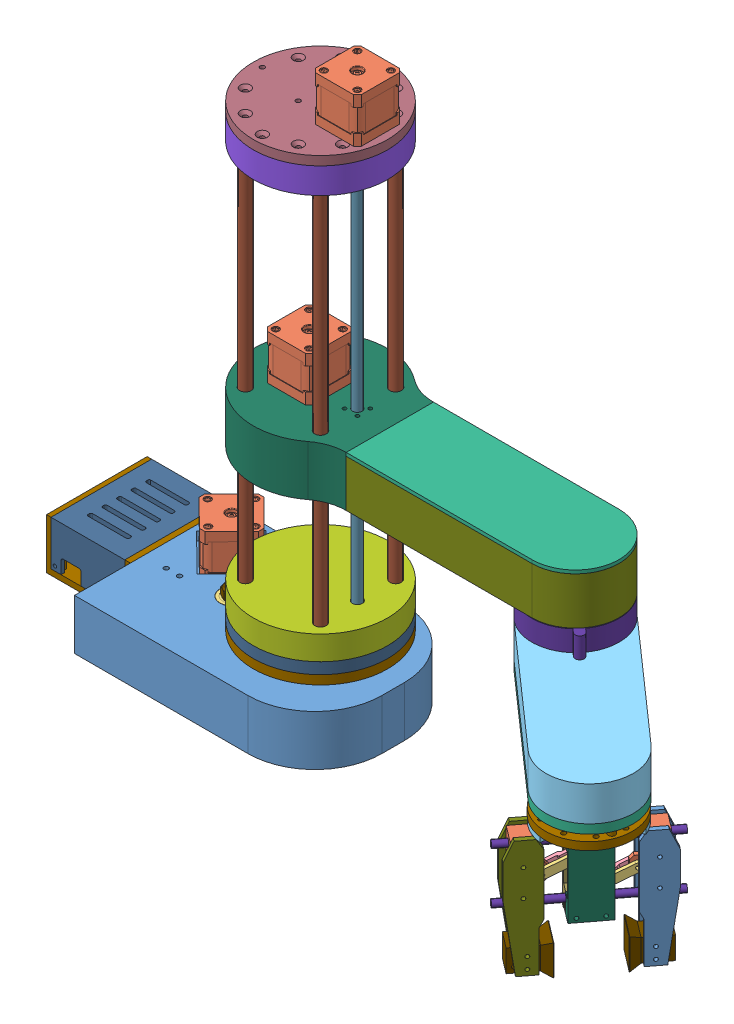
SolidWorks assembly SCARA Robot, configuration SCARA Robot. Lengths in mm.
Overall size (616.01 508 221.86).
112 component instances, 59 part files, 217 mates.
Components (placement in the parent):
- Base-1: Base [Base] at origin size (215 45 140)
- Stepper NEMA 17 -  20mm shaft-1: Stepper NEMA 17 -  20mm shaft [Stepper NEMA 17 -  20mm shaft] at (-89.369 63.0261 0.1561) x (-0.712104 0 -0.702074) z (0 -1 0) size (41 41 60)
- Ball Bearing 608 - 8x22x7mm-2: Ball Bearing 608 - 8x22x7mm [Ball Bearing 608 - 8x22x7mm] at (-36.5 3 0) x (0.982643 0 -0.185507) z (0.185507 0 0.982643) size (22 7 22)
- Ball Bearing 608 - 8x22x7mm-3: Ball Bearing 608 - 8x22x7mm [Ball Bearing 608 - 8x22x7mm] at (-36.5 -7.5 0) x (0.997797 0 -0.066338) z (0.066338 0 0.997797) size (22 7 22)
- Thrust Bearing - 40x60x13-3: Thrust Bearing - 40x60x13 [Thrust Bearing - 40x60x13] at (42.5 -13 0) size (60 13 60)
- Thrust Bearing - 40x60x13-4: Thrust Bearing - 40x60x13 [Thrust Bearing - 40x60x13] at (42.5 10 0) x (0.998314 0 0.058039) z (-0.058039 0 0.998314) size (60 13 60)
- GT2 Pulley - 110 teeth - J1-2: GT2 Pulley - 110 teeth - J1 [GT2 Pulley - Parametric] at (42.5 -11.2 0) x (-1 0 0) z (0 0 1) size (71.92 22.4 71.92)
- GT2 Pulley - 22 - 80 teeth-2: GT2 Pulley - 22 - 80 teeth [GT2 Pulley - Parametric] at (-36.5 -26.3 0) x (0.998061 0 0.062248) z (-0.062248 0 0.998061) size (52.82 18.8 52.82)
- GT2 Pulley - Parametric-1: GT2 Pulley - Parametric [GT2 Pulley - Parametric] at (-69.2568 -19.3 -32.2954) x (-0.837169 0 -0.546944) z (-0.546944 0 0.837169) size (14.62 15.2 14.62)
- M8 Washer-2: M8 Washer [M8 Washer] at (-36.5 -8.7 0) x (0.759776 0 0.650185) z (-0.650185 0 0.759776) size (14 1.2 14)
- J1 coupler-1: J1 coupler [J1 coupler] at (42.5 23 0) x (0 0 1) z (-1 0 0) size (120 27 120)
- Z-axis Bottom Plate-2: Z-axis Bottom Plate [Z-axis Bottom Plate] at (42.5 31 0) x (0 0 -1) z (1 0 0) size (120 10 120)
- Smooth Rod D10mm L400mm-1: Smooth Rod D10mm L400mm [Smooth Rod D10mm L400mm] at (76.0876 25 -33.5876) x (-0.2209 0 0.975296) z (-0.975296 0 -0.2209) size (10 400 10)
- Smooth Rod D10mm L400mm-2: Smooth Rod D10mm L400mm [Smooth Rod D10mm L400mm] at (76.0876 25 33.5876) size (10 400 10)
- Smooth Rod D10mm L400mm-3: Smooth Rod D10mm L400mm [Smooth Rod D10mm L400mm] at (8.9124 25 33.5876) size (10 400 10)
- Smooth Rod D10mm L400mm-4: Smooth Rod D10mm L400mm [Smooth Rod D10mm L400mm] at (8.9124 25 -33.5876) size (10 400 10)
- Smooth Rod Clamp-1: Smooth Rod Clamp [Smooth Rod Clamp] at (76.0876 41 33.5876) x (0.707107 0 -0.707107) z (0.707107 0 0.707107) size (39.1 14 26.4)
- Smooth Rod Clamp-2: Smooth Rod Clamp [Smooth Rod Clamp] at (8.9124 41 33.5876) x (0.707107 0 0.707107) z (-0.707107 0 0.707107) size (39.1 14 26.4)
- Smooth Rod Clamp-3: Smooth Rod Clamp [Smooth Rod Clamp] at (8.9124 41 -33.5876) x (-0.707107 0 0.707107) z (-0.707107 0 -0.707107) size (39.1 14 26.4)
- Smooth Rod Clamp-4: Smooth Rod Clamp [Smooth Rod Clamp] at (76.0876 41 -33.5876) x (-0.707107 0 -0.707107) z (0.707107 0 -0.707107) size (39.1 14 26.4)
- Z-axis Top Plate-1: Z-axis Top Plate [Z-axis Top Plate] at (42.5 425 0) x (0 0 -1) z (1 0 0) size (120 26 120)
- Smooth Rod Clamp-5: Smooth Rod Clamp [Smooth Rod Clamp] at (8.9124 411 33.5876) x (0.707107 0 0.707107) z (-0.707107 0 0.707107) size (39.1 14 26.4)
- Smooth Rod Clamp-6: Smooth Rod Clamp [Smooth Rod Clamp] at (76.0876 411 33.5876) x (0.707107 0 -0.707107) z (0.707107 0 0.707107) size (39.1 14 26.4)
- Smooth Rod Clamp-7: Smooth Rod Clamp [Smooth Rod Clamp] at (76.0876 411 -33.5876) x (-0.707107 0 -0.707107) z (0.707107 0 -0.707107) size (39.1 14 26.4)
- Smooth Rod Clamp-8: Smooth Rod Clamp [Smooth Rod Clamp] at (8.9124 411 -33.5876) x (-0.707107 0 0.707107) z (-0.707107 0 -0.707107) size (39.1 14 26.4)
- Lead Screw D8mm L380mm-1: Lead Screw D8mm L380mm [Lead Screw D8mm L380mm] at (75.5 33 0) x (0.999653 0 0.026358) z (-0.026358 0 0.999653) size (8 380 8)
- Ball Bearing 608 - 8x22x7mm-4: Ball Bearing 608 - 8x22x7mm [Ball Bearing 608 - 8x22x7mm] at (75.5 34 0) x (0.948058 0 -0.318097) z (0.318097 0 0.948058) size (22 7 22)
- Stepper NEMA 17 -  20mm shaft-2: Stepper NEMA 17 -  20mm shaft [Stepper NEMA 17 -  20mm shaft] at (38.2709 494.0261 8.4614) x (0 0 -1) z (0 -1 0) size (41 41 60)
- Z-axis Mount Platform-1: Z-axis Mount Platform [Z-axis Mount Platform] at (42.5 211.1984 0) x (0 0 1) z (1 0 0) size (120 45 122)
- Arm 1-1: Arm 1 [Arm 1] at (270.5 166.1984 0) size (205 42 78)
- Ball Bearing 608 - 8x22x7mm-5: Ball Bearing 608 - 8x22x7mm [Ball Bearing 608 - 8x22x7mm] at (180.5 182.1984 0) x (0.62791 0 0.778286) z (0.778286 0 -0.62791) size (22 7 22)
- Ball Bearing 608 - 8x22x7mm-6: Ball Bearing 608 - 8x22x7mm [Ball Bearing 608 - 8x22x7mm] at (180.5 173.1984 0) x (0.619443 0 0.785042) z (0.785042 0 -0.619443) size (22 7 22)
- J2 Coupler-1: J2 Coupler [J2 Coupler] at (270.5 147.1984 0) x (0.198234 0 -0.980155) z (0.980155 0 0.198234) size (78 24 80.24)
- Thrust Bearing 35x52x12mm-1: Thrust Bearing 35x52x12mm [Thrust Bearing 35x52x12mm] at (270.5 154.1984 0) x (1 0 0.000333) z (-0.000333 0 1) size (52 12 52)
- Ball Bearing 30x42x7mm-1: Ball Bearing 30x42x7mm [Ball Bearing 30x42x7mm] at (270.5 169.1984 0) x (1 0 0.000333) z (-0.000333 0 1) size (42 7 42)
- GT2 Pulley - 92 teeth - J2-1: GT2 Pulley - 92 teeth - J2 [GT2 Pulley - Parametric] at (270.5 184.3984 0) x (0.980155 0 0.198234) z (-0.198234 0 0.980155) size (60.46 20.4 60.46)
- GT2 Pulley - 23 - 80 teeth-1: GT2 Pulley - 23 - 80 teeth [GT2 Pulley - Parametric] at (180.5 200.9984 0) x (-0.873164 0 -0.487427) z (-0.487427 0 0.873164) size (52.82 18.8 52.82)
- Thrust Bearing 35x52x12mm-2: Thrust Bearing 35x52x12mm [Thrust Bearing 35x52x12mm] at (270.5 176.1984 0) x (1 0 0.000333) z (-0.000333 0 1) size (52 12 52)
- Stepper NEMA 17 -  20mm shaft-3: Stepper NEMA 17 -  20mm shaft [Stepper NEMA 17 -  20mm shaft] at (-4.7291 272.2245 8.4614) x (0 0 -1) z (0 -1 0) size (41 41 60)
- GT2 Pulley - Parametric-2: GT2 Pulley - Parametric [GT2 Pulley - Parametric] at (32.5 200.9984 0) x (-0.529245 0 -0.848469) z (-0.848469 0 0.529245) size (14.62 15.2 14.62)
- M8 Washer-3: M8 Washer [M8 Washer] at (180.5 182.1984 0) x (0.759776 0 0.650185) z (-0.650185 0 0.759776) size (14 1.2 14)
- Linear Bearing 10x19x29mm-1: Linear Bearing 10x19x29mm [Linear Bearing 10x19x29mm] at (8.9124 176.1984 -33.5876) x (0.996362 0 -0.085221) z (0.085221 0 0.996362) size (19 29 19)
- Linear Bearing 10x19x29mm-2: Linear Bearing 10x19x29mm [Linear Bearing 10x19x29mm] at (76.0876 176.1984 -33.5876) x (0.940518 0 0.339744) z (-0.339744 0 0.940518) size (19 29 19)
- Linear Bearing 10x19x29mm-3: Linear Bearing 10x19x29mm [Linear Bearing 10x19x29mm] at (8.9124 176.1984 33.5876) size (19 29 19)
- Linear Bearing 10x19x29mm-6: Linear Bearing 10x19x29mm [Linear Bearing 10x19x29mm] at (76.0876 176.1984 33.5876) size (19 29 19)
- Arm 2-1: Arm 2 [Arm 2] at (378.46 147.1984 95.2924) x (0.749722 0 0.661753) z (0.661753 0 -0.749722) size (222 31 78)
- Arm 2 Cover-1: Arm 2 Cover [Arm 2 Cover] at (378.46 108.1984 95.2924) x (0.749722 0 0.661753) z (-0.661753 0 0.749722) size (222 8 78)
- Micro switch-1: Micro switch [Micro switch] at (217.6469 166.1984 9.5547) x (0.882948 0 -0.469472) z (0 -1 0) size (21.91 25.05 6)
- NEMA 17 Stepper L24mm - 20mm shaft-1: NEMA 17 Stepper L24mm - 20mm shaft [NEMA 17 Stepper L24mm - 20mm shaft] at (266.0017 84.1984 -3.9705) x (0.749722 0 0.661753) z (-0.661753 0 0.749722) size (42 46 42)
- J3 Coupler-1: J3 Coupler [J3 Coupler] at (372.8371 90.1984 90.3293) x (-0.943757 0 -0.330639) z (0.330639 0 -0.943757) size (77.59 22 78)
- Ball Bearing 30x42x7mm-2: Ball Bearing 30x42x7mm [Ball Bearing 30x42x7mm] at (372.8371 116.1984 90.3293) x (-0.837351 0 -0.546665) z (-0.546665 0 0.837351) size (42 7 42)
- Thrust Bearing 35x52x12mm-3: Thrust Bearing 35x52x12mm [Thrust Bearing 35x52x12mm] at (372.8371 116.1984 90.3293) x (0.88853 0 -0.458819) z (0.458819 0 0.88853) size (52 12 52)
- Thrust Bearing 35x52x12mm-4: Thrust Bearing 35x52x12mm [Thrust Bearing 35x52x12mm] at (372.8371 108.1984 90.3293) x (-0.531744 0 -0.846905) z (-0.846905 0 0.531744) size (52 12 52)
- GT2 Pulley - 90 teeth - J3-1: GT2 Pulley - 90 teeth - J3 [GT2 Pulley - Parametric] at (372.8371 126.3984 90.3293) x (-0.330639 0 0.943757) z (-0.943757 0 -0.330639) size (59.19 21.4 59.19)
- GT2 Pulley - Parametric-3: GT2 Pulley - Parametric [GT2 Pulley - Parametric] at (266.0017 126.3984 -3.9705) x (0.907133 0 -0.420845) z (0.420845 0 0.907133) size (14.62 15.2 14.62)
- Micro switch-3: Micro switch [Micro switch] at (-8.7411 16 2.5547) x (0.882948 0 -0.469472) z (0 -1 0) size (21.91 25.05 6)
- Micro switch-4: Micro switch [Micro switch] at (333.7206 108.1984 68.5469) x (0.972639 0 0.23232) z (0 -1 0) size (21.91 25.05 6)
- Lead Screw Nut 8mm-1: Lead Screw Nut 8mm [Lead Screw Nut 8mm] at (75.5 201.6984 0) size (22 15 22)
- Gripper Mechanism-1: Gripper Mechanism [Gripper Mechanism] at (318.5346 102.8101 87.5004) x (0.606093 0 -0.795394) z (0 -1 0) size (125 124.2 111.5)
  - Servo Holder-1: Servo Holder [Servo Holder] at (30.6623 30.9064 53.3617) size (44 15 72.5)
  - Servo Motor MG996R 3D Model-1: Servo Motor MG996R 3D Model [Servo Motor MG996R 3D Model] at (30.6623 -0.2936 62.3617) x (0 0 1) z (-1 0 0) size (55.8 45.2 20.5)
  - Servo MG996R Horn-1: Servo MG996R Horn [Servo MG996R Horn] at (30.6623 44.9064 52.1117) x (0.468503 0 0.883462) z (-0.883462 0 0.468503) size (32 2.5 12)
  - Gripper Cover-1: Gripper Cover [Gripper Cover] at (30.6623 56.4064 52.1117) x (-1 0 0) z (0 0 1) size (44 10.5 70)
  - Gripper Hand Left-1: Gripper Hand Left [Gripper Hand Left] at (0.1145 53.9064 27.1117) size (26 4 105)
  - Gripper rail 6mm-1: Gripper rail 6mm [Gripper rail 6mm] at (-31.8377 44.9064 75.1117) x (0 0.568693 0.82255) z (0 0.82255 -0.568693) size (6 125 6)
  - Gripper End-1: Gripper End [Gripper End] at (-23.3855 44.9064 114.1117) x (0 0 1) z (0 1 0) size (27.12 30 25.12)
  - Gripper Hand Right-1: Gripper Hand Right [Gripper Hand Left] at (61.21 53.9064 27.1117) size (26 4 105)
  - Gripper rail 6mm-2: Gripper rail 6mm [Gripper rail 6mm] at (93.1623 44.9064 29.1117) x (0 0.838695 -0.544602) z (0 0.544602 0.838695) size (6 125 6)
  - Gripper Mechanism Slider-3: Gripper Mechanism Slider [Gripper Mechanism Slider] at (-20.8855 44.9064 52.1117) x (0 1 0) z (0 0 -1) size (18 26 60)
  - Gripper Mechanism Slider-4: Gripper Mechanism Slider [Gripper Mechanism Slider] at (82.21 44.9064 52.1117) x (0 -1 0) z (0 0 -1) size (18 26 60)
  - Gripper Hand Left-2: Gripper Hand Left [Gripper Hand Left] at (0.1145 31.9064 27.1117) size (26 4 105)
  - Gripper Hand Right-2: Gripper Hand Right [Gripper Hand Left] at (61.21 31.9064 27.1117) size (26 4 105)
  - Gripper End-2: Gripper End [Gripper End] at (84.71 44.9064 114.1117) x (0 0 -1) z (0 1 0) size (27.12 30 25.12)
  - Gripper link 1-1: Gripper link 1 [Gripper link 1] at (24.3375 47.4064 40.185) x (0.897148 0 -0.441731) z (0.441731 0 0.897148) size (34.2 3.5 7.2)
  - Gripper link 2-1: Gripper link 2 [Gripper link 2] at (0.1145 39.9064 52.1117) x (-0.897148 0 0.441731) z (-0.441731 0 -0.897148) size (34.2 5 7.2)
  - Gripper link 1-2: Gripper link 1 [Gripper link 1] at (61.21 47.4064 52.1117) x (0.897148 0 -0.441731) z (0.441731 0 0.897148) size (34.2 3.5 7.2)
  - Gripper link 2-2: Gripper link 2 [Gripper link 2] at (36.9871 44.9064 64.0385) x (-0.897148 0 0.441731) z (0.441731 0 0.897148) size (34.2 5 7.2)
  - Gripper to J3 connector-1: Gripper to J3 connector [Gripper to J3 connector] at (30.6623 44.9064 17.1117) x (0 -1 0) z (1 0 0) size (39 4.5 78)
  - Wide gripper end-1: Wide gripper end [Wide gripper end] at (-15.3855 35.9064 114.1117) x (1 0 0) z (0 1 0) size (24 20 88) (hidden)
  - Wide gripper end - Left side-1: Wide gripper end - Left side [Wide gripper end - Left side] at (76.71 35.9064 114.1117) x (1 0 0) z (0 1 0) size (24 20 88) (hidden)
- Arm 1 Cover-1: Arm 1 Cover [Arm 1 Cover] at (270.5 211.1984 0) x (1 0 0) z (0 0 -1) size (205 11 78)
- Micro switch-5: Micro switch [Micro switch] at (14.25 412 6) x (1 0 0) z (0 0 -1) size (21.91 25.05 6)
- Base cover-1: Base cover [Base cover] at (42.5 62.5 0) x (1 0 0) z (0 0 -1) size (120 21.5 120)
- Top cover-1: Top cover [Top cover] at (42.5 402 0) size (120 23 120)
- Arduino UNO case p1-1: Arduino UNO case p1 [Arduino UNO case p1] at (-145 -32.5 -70) size (75 45 90)
- Arduino UNO case p2-1: Arduino UNO case p2 [Arduino UNO case p2] at (-145.5 8 -70) size (66 40 90)
- GT2 Belt 200mm-1: GT2 Belt 200mm [GT2 Belt 400mm] at (-36.5 -25.3 0) x (0.712104 0 0.702074) z (-0.702074 0 0.712104) size (79.45 6 52.6)
- GT2 Belt 300mm 2-1: GT2 Belt 300mm 2 [GT2 Belt 400mm] at (42.5 -17.2 0) size (122.6 6 71.6)
- GT2 Belt 400mm-1: GT2 Belt 400mm [GT2 Belt 400mm] at (180.5 194.9984 0) size (181.45 6 52.6)
- GT2 Belt 300mm-1: GT2 Belt 300mm [GT2 Belt 400mm] at (270.5 185.3984 0) size (128.2 6 60.2)
- GT2 Belt 400mm 2-1: GT2 Belt 400mm 2 [GT2 Belt 400mm] at (372.8371 126.3984 90.3293) x (0.749722 0 0.661753) z (-0.661753 0 0.749722) size (179.1 6 58.9)
- Ball Bearing 35x47x7mm-1: Ball Bearing 35x47x7mm [Ball Bearing 30x42x7mm] at (42.5 0 0) x (0.999968 0 0.008039) z (-0.008039 0 0.999968) size (47 7 47)
- M8 45mm - Bolts-1: M8 45mm - Bolts [M8 45mm - Bolts] at (-36.5 -7.65 0) x (0 1 0) z (-0.873774 0 -0.486332) size (50.3 15.01 13)
- M8 Lock nut-1: M8 Lock nut [M8 Lock nut] at (-36.5 10 0) x (-0.45229 0 0.891871) z (-0.891871 0 -0.45229) size (13 8 15.01)
- M8 45mm - Bolts-3: M8 45mm - Bolts [M8 45mm - Bolts] at (180.5 182.3484 0) x (0 -1 0) z (0.786055 0 0.618156) size (50.3 15.01 13)
- M8 Lock nut-3: M8 Lock nut [M8 Lock nut] at (180.5 166.1984 0) x (-0.837169 0 -0.546944) z (-0.546944 0 0.837169) size (13 8 15.01)
- M4 Lock nut-1: M4 Lock nut [M4 Lock nut] at (259.7183 192.5984 -2.1806) size (7 5 8.08)
- M4 Lock nut-2: M4 Lock nut [M4 Lock nut] at (272.6806 192.5984 -10.7817) size (7 5 8.08)
- M4 Lock nut-3: M4 Lock nut [M4 Lock nut] at (281.2817 192.5984 2.1806) size (7 5 8.08)
- M4 Lock nut-4: M4 Lock nut [M4 Lock nut] at (268.3194 192.5984 10.7817) size (7 5 8.08)
- M4 60mm - Bolts-1: M4 60mm - Bolts [M4 60mm - Bolts] at (42.5 28.8 -12.5) x (-0.292697 0 -0.956205) z (0 1 0) size (7.5 7.5 60)
- M4 60mm - Bolts-2: M4 60mm - Bolts [M4 60mm - Bolts] at (30 28.8 0) x (1 0 0) z (0 1 0) size (7.5 7.5 60)
- M4 60mm - Bolts-3: M4 60mm - Bolts [M4 60mm - Bolts] at (55 28.8 0) x (1 0 0) z (0 1 0) size (7.5 7.5 60)
- M4 60mm - Bolts-4: M4 60mm - Bolts [M4 60mm - Bolts] at (42.5 28.8 12.5) x (1 0 0) z (0 1 0) size (7.5 7.5 60)
- M4 50mm - Bolts-1: M4 50mm - Bolts [M4 50mm - Bolts] at (259.7183 149.3984 -2.1806) x (1 0 0) z (0 -1 0) size (7.5 7.5 50)
- M4 50mm - Bolts-2: M4 50mm - Bolts [M4 50mm - Bolts] at (268.3194 149.3984 10.7817) x (1 0 0) z (0 -1 0) size (7.5 7.5 50)
- M4 50mm - Bolts-3: M4 50mm - Bolts [M4 50mm - Bolts] at (281.2817 149.3984 2.1806) x (1 0 0) z (0 -1 0) size (7.5 7.5 50)
- M4 50mm - Bolts-4: M4 50mm - Bolts [M4 50mm - Bolts] at (272.6806 149.3984 -10.7817) x (1 0 0) z (0 -1 0) size (7.5 7.5 50)
- M4 Lock nut-5: M4 Lock nut [M4 Lock nut] at (42.5 -19.4 12.5) x (-0.837169 0 -0.546944) z (-0.546944 0 0.837169) size (7 5 8.08)
- M4 Lock nut-6: M4 Lock nut [M4 Lock nut] at (42.5 -19.4 -12.5) x (-0.837169 0 -0.546944) z (-0.546944 0 0.837169) size (7 5 8.08)
- M4 Lock nut-7: M4 Lock nut [M4 Lock nut] at (55 -19.4 0) x (-0.837169 0 -0.546944) z (-0.546944 0 0.837169) size (7 5 8.08)
- M4 Lock nut-8: M4 Lock nut [M4 Lock nut] at (30 -19.4 0) x (-0.837169 0 -0.546944) z (-0.546944 0 0.837169) size (7 5 8.08)
Mates (geometry in assembly coordinates):
- Concentric1: concentric aligned: cylinder of Base-1 through (-69.2568 0 -32.2954) axis (0 1 0) radius 12.5; cylinder of Stepper NEMA 17 -  20mm shaft-1 through (-69.2568 0.01 -32.2954) axis (0 1 0) radius 11.5
- Parallel1: parallel anti-aligned: plane of Base-1 through (-69.0361 2 -1.1835) normal (0.702074 0 -0.712104); plane of Stepper NEMA 17 -  20mm shaft-1 through (-71.5435 2 -5.762) normal (-0.702074 0 0.712104)
- Coincident2: coincident anti-aligned: plane of Base-1 through (0 2 0) normal (0 1 0); plane of Stepper NEMA 17 -  20mm shaft-1 through (-83.6493 2 -17.6973) normal (0 -1 0)
- Concentric2: concentric anti-aligned: cylinder of Base-1 through (-36.5 3 0) axis (0 1 0) radius 11; cylinder of Ball Bearing 608 - 8x22x7mm-2 through (-36.5 10 0) axis (0 -1 0) radius 11
- Coincident3: coincident anti-aligned: plane of Base-1 through (-36.5 3 0) normal (0 1 0); plane of Ball Bearing 608 - 8x22x7mm-2 through (-36.5 3 0) normal (0 -1 0)
- Concentric3: concentric anti-aligned: cylinder of Base-1 through (-36.5 -8.5 0) axis (0 1 0) radius 11; cylinder of Ball Bearing 608 - 8x22x7mm-3 through (-36.5 -0.5 0) axis (0 -1 0) radius 11
- Concentric4: concentric aligned: cylinder of Base-1 through (42.5 0 0) axis (0 1 0) radius 20; cylinder of Thrust Bearing - 40x60x13-4 through (42.5 19.2 0) axis (0 1 0) radius 30
- Coincident5: coincident anti-aligned: plane of Base-1 through (0 10 0) normal (0 1 0); plane of Thrust Bearing - 40x60x13-4 through (42.5 10 0) normal (0 -1 0)
- Concentric5: concentric anti-aligned: cylinder of Base-1 through (42.5 -8 0) axis (0 1 0) radius 30.5; cylinder of Thrust Bearing - 40x60x13-3 through (42.5 -9.2 0) axis (0 -1 0) radius 30
- Coincident6: coincident anti-aligned: plane of Base-1 through (0 0 0) normal (0 -1 0); plane of Thrust Bearing - 40x60x13-3 through (42.5 0 0) normal (0 1 0)
- Concentric6: concentric anti-aligned: cylinder of Ball Bearing 608 - 8x22x7mm-3 through (-36.5 -0.5 0) axis (0 -1 0) radius 4; cylinder of GT2 Pulley - 22 - 80 teeth-2 through (-36.5 -27.5 0) axis (0 1 0) radius 4
- Concentric7: concentric aligned: cylinder of Ball Bearing 608 - 8x22x7mm-3 through (-36.5 -0.5 0) axis (0 -1 0) radius 4; cylinder of M8 Washer-2 through (-36.5 -7.5 0) axis (0 -1 0) radius 7
- Coincident7: coincident anti-aligned: plane of Ball Bearing 608 - 8x22x7mm-3 through (-36.5 -7.5 0) normal (0 -1 0); plane of M8 Washer-2 through (-36.5 -7.5 0) normal (0 1 0)
- Coincident8: coincident anti-aligned: plane of GT2 Pulley - 22 - 80 teeth-2 through (-36.5 -8.7 0) normal (0 1 0); plane of M8 Washer-2 through (-36.5 -8.7 0) normal (0 -1 0)
- Concentric8: concentric anti-aligned: cylinder of Thrust Bearing - 40x60x13-3 through (42.5 -3.8 0) axis (0 1 0) radius 20; cylinder of GT2 Pulley - 110 teeth - J1-2 through (42.5 3 0) axis (0 -1 0) radius 17.5
- Coincident9: coincident anti-aligned: plane of Thrust Bearing - 40x60x13-3 through (42.5 -13 0) normal (0 -1 0); plane of GT2 Pulley - 110 teeth - J1-2 through (42.5 -13 0) normal (0 1 0)
- Concentric9: concentric anti-aligned: cylinder of Stepper NEMA 17 -  20mm shaft-1 through (-69.2568 -20 -32.2954) axis (0 1 0) radius 2.5; cylinder of GT2 Pulley - Parametric-1 through (-69.2568 -12.3 -32.2954) axis (0 -1 0) radius 2.5
- Coincident10: coincident aligned: plane of GT2 Pulley - 22 - 80 teeth-2 through (-36.5 -19.3 0) normal (0 -1 0); plane of GT2 Pulley - Parametric-1 through (-69.2568 -19.3 -32.2954) normal (0 -1 0)
- Coincident11: coincident anti-aligned: plane of Thrust Bearing - 40x60x13-4 through (42.5 23 0) normal (0 1 0); plane of J1 coupler-1 through (42.5 23 0) normal (0 -1 0)
- Concentric10: concentric aligned: cylinder of Thrust Bearing - 40x60x13-4 through (42.5 18.2 0) axis (0 -1 0) radius 30; cylinder of J1 coupler-1 through (42.5 31 0) axis (0 -1 0) radius 60
- Concentric11: concentric anti-aligned: cylinder of GT2 Pulley - 110 teeth - J1-2 through (55 3 0) axis (0 -1 0) radius 1.8; cylinder of J1 coupler-1 through (55 31 0) axis (0 1 0) radius 1.8
- Coincident13: coincident anti-aligned: plane of Base-1 through (-36.5 -0.5 0) normal (0 -1 0); plane of Ball Bearing 608 - 8x22x7mm-3 through (-36.5 -0.5 0) normal (0 1 0)
- Concentric12: concentric anti-aligned: cylinder of J1 coupler-1 through (76.0876 23 -33.5876) axis (0 1 0) radius 4.975; cylinder of Smooth Rod D10mm L400mm-1 through (76.0876 425 -33.5876) axis (0 -1 0) radius 5
- Coincident14: coincident anti-aligned: plane of J1 coupler-1 through (76.0876 25 -33.5876) normal (0 1 0); plane of Smooth Rod D10mm L400mm-1 through (76.0876 25 -33.5876) normal (0 -1 0)
- Concentric13: concentric anti-aligned: cylinder of J1 coupler-1 through (8.9124 23 -33.5876) axis (0 1 0) radius 4.975; cylinder of Smooth Rod D10mm L400mm-4 through (8.9124 425 -33.5876) axis (0 -1 0) radius 5
- Concentric14: concentric anti-aligned: cylinder of J1 coupler-1 through (8.9124 23 33.5876) axis (0 1 0) radius 4.975; cylinder of Smooth Rod D10mm L400mm-3 through (8.9124 425 33.5876) axis (0 -1 0) radius 5
- Concentric15: concentric anti-aligned: cylinder of J1 coupler-1 through (76.0876 23 33.5876) axis (0 1 0) radius 4.975; cylinder of Smooth Rod D10mm L400mm-2 through (76.0876 425 33.5876) axis (0 -1 0) radius 5
- Coincident15: coincident aligned: plane of Smooth Rod D10mm L400mm-1 through (76.0876 425 -33.5876) normal (0 1 0); plane of Smooth Rod D10mm L400mm-2 through (76.0876 425 33.5876) normal (0 1 0)
- Coincident16: coincident aligned: plane of Smooth Rod D10mm L400mm-1 through (76.0876 425 -33.5876) normal (0 1 0); plane of Smooth Rod D10mm L400mm-3 through (8.9124 425 33.5876) normal (0 1 0)
- Coincident17: coincident aligned: plane of Smooth Rod D10mm L400mm-1 through (76.0876 425 -33.5876) normal (0 1 0); plane of Smooth Rod D10mm L400mm-4 through (8.9124 425 -33.5876) normal (0 1 0)
- Concentric16: concentric aligned: cylinder of J1 coupler-1 through (42.5 31 0) axis (0 -1 0) radius 60; cylinder of Z-axis Bottom Plate-2 through (42.5 41 0) axis (0 -1 0) radius 60
- Concentric17: concentric anti-aligned: cylinder of Z-axis Bottom Plate-2 through (76.0876 31 -33.5876) axis (0 1 0) radius 4.975; cylinder of Smooth Rod D10mm L400mm-1 through (76.0876 425 -33.5876) axis (0 -1 0) radius 5
- Coincident18: coincident anti-aligned: plane of J1 coupler-1 through (42.5 31 0) normal (0 1 0); plane of Z-axis Bottom Plate-2 through (42.5 31 0) normal (0 -1 0)
- Concentric18: concentric aligned: cylinder of Smooth Rod D10mm L400mm-2 through (76.0876 425 33.5876) axis (0 -1 0) radius 5; cylinder of Smooth Rod Clamp-1 through (76.0876 55 33.5876) axis (0 -1 0) radius 5
- Concentric19: concentric anti-aligned: cylinder of Z-axis Bottom Plate-2 through (66.1881 31 43.4871) axis (0 1 0) radius 2.05; cylinder of Smooth Rod Clamp-1 through (66.1881 55 43.4871) axis (0 -1 0) radius 2.05
- Coincident19: coincident anti-aligned: plane of Z-axis Bottom Plate-2 through (42.5 41 0) normal (0 1 0); plane of Smooth Rod Clamp-1 through (66.1881 41 43.4871) normal (0 -1 0)
- Coincident20: coincident anti-aligned: plane of Z-axis Bottom Plate-2 through (42.5 41 0) normal (0 1 0); plane of Smooth Rod Clamp-4 through (85.9871 41 -23.6881) normal (0 -1 0)
- Concentric20: concentric aligned: cylinder of Smooth Rod D10mm L400mm-1 through (76.0876 425 -33.5876) axis (0 -1 0) radius 5; cylinder of Smooth Rod Clamp-4 through (76.0876 55 -33.5876) axis (0 -1 0) radius 5
- Concentric21: concentric anti-aligned: cylinder of Z-axis Bottom Plate-2 through (66.1881 31 -43.4871) axis (0 1 0) radius 2.05; cylinder of Smooth Rod Clamp-4 through (66.1881 55 -43.4871) axis (0 -1 0) radius 2.05
- Coincident21: coincident anti-aligned: plane of Z-axis Bottom Plate-2 through (42.5 41 0) normal (0 1 0); plane of Smooth Rod Clamp-2 through (-0.9871 41 23.6881) normal (0 -1 0)
- Concentric22: concentric aligned: cylinder of Smooth Rod D10mm L400mm-3 through (8.9124 425 33.5876) axis (0 -1 0) radius 5; cylinder of Smooth Rod Clamp-2 through (8.9124 55 33.5876) axis (0 -1 0) radius 5
- Concentric23: concentric anti-aligned: cylinder of Z-axis Bottom Plate-2 through (18.8119 31 43.4871) axis (0 1 0) radius 2.05; cylinder of Smooth Rod Clamp-2 through (18.8119 55 43.4871) axis (0 -1 0) radius 2.05
- Concentric24: concentric aligned: cylinder of Smooth Rod D10mm L400mm-4 through (8.9124 425 -33.5876) axis (0 -1 0) radius 5; cylinder of Smooth Rod Clamp-3 through (8.9124 55 -33.5876) axis (0 -1 0) radius 5
- Concentric25: concentric anti-aligned: cylinder of Z-axis Bottom Plate-2 through (-0.9871 31 -23.6881) axis (0 1 0) radius 2.05; cylinder of Smooth Rod Clamp-3 through (-0.9871 55 -23.6881) axis (0 -1 0) radius 2.05
- Coincident22: coincident anti-aligned: plane of Z-axis Bottom Plate-2 through (42.5 41 0) normal (0 1 0); plane of Smooth Rod Clamp-3 through (18.8119 41 -43.4871) normal (0 -1 0)
- Coincident23: coincident anti-aligned: plane of Z-axis Top Plate-1 through (42.5 425 0) normal (0 -1 0); plane of Smooth Rod Clamp-6 through (66.1881 425 43.4871) normal (0 1 0)
- Concentric26: concentric anti-aligned: cylinder of Z-axis Top Plate-1 through (85.9871 425 23.6881) axis (0 1 0) radius 2.05; cylinder of Smooth Rod Clamp-6 through (85.9871 425 23.6881) axis (0 -1 0) radius 2.05
- Concentric27: concentric anti-aligned: cylinder of Z-axis Top Plate-1 through (66.1881 425 43.4871) axis (0 1 0) radius 2.05; cylinder of Smooth Rod Clamp-6 through (66.1881 425 43.4871) axis (0 -1 0) radius 2.05
- Coincident24: coincident anti-aligned: plane of Z-axis Top Plate-1 through (42.5 425 0) normal (0 -1 0); plane of Smooth Rod Clamp-8 through (18.8119 425 -43.4871) normal (0 1 0)
- Concentric28: concentric anti-aligned: cylinder of Z-axis Top Plate-1 through (18.8119 425 -43.4871) axis (0 1 0) radius 2.05; cylinder of Smooth Rod Clamp-8 through (18.8119 425 -43.4871) axis (0 -1 0) radius 2.05
- Concentric29: concentric anti-aligned: cylinder of Z-axis Top Plate-1 through (-0.9871 425 -23.6881) axis (0 1 0) radius 2.05; cylinder of Smooth Rod Clamp-8 through (-0.9871 425 -23.6881) axis (0 -1 0) radius 2.05
- Coincident25: coincident anti-aligned: plane of Z-axis Top Plate-1 through (42.5 425 0) normal (0 -1 0); plane of Smooth Rod Clamp-7 through (85.9871 425 -23.6881) normal (0 1 0)
- Concentric32: concentric anti-aligned: cylinder of Z-axis Top Plate-1 through (66.1881 425 -43.4871) axis (0 1 0) radius 2.05; cylinder of Smooth Rod Clamp-7 through (66.1881 425 -43.4871) axis (0 -1 0) radius 2.05
- Concentric33: concentric anti-aligned: cylinder of Z-axis Top Plate-1 through (85.9871 425 -23.6881) axis (0 1 0) radius 2.05; cylinder of Smooth Rod Clamp-7 through (85.9871 425 -23.6881) axis (0 -1 0) radius 2.05
- Coincident26: coincident anti-aligned: plane of Z-axis Top Plate-1 through (42.5 425 0) normal (0 -1 0); plane of Smooth Rod Clamp-5 through (-0.9871 425 23.6881) normal (0 1 0)
- Concentric34: concentric anti-aligned: cylinder of Z-axis Top Plate-1 through (-0.9871 425 23.6881) axis (0 1 0) radius 2.05; cylinder of Smooth Rod Clamp-5 through (-0.9871 425 23.6881) axis (0 -1 0) radius 2.05
- Concentric35: concentric anti-aligned: cylinder of Z-axis Top Plate-1 through (18.8119 425 43.4871) axis (0 1 0) radius 2.05; cylinder of Smooth Rod Clamp-5 through (18.8119 425 43.4871) axis (0 -1 0) radius 2.05
- Concentric36: concentric aligned: cylinder of Z-axis Bottom Plate-2 through (75.5 34 0) axis (0 1 0) radius 11; cylinder of Z-axis Top Plate-1 through (75.5 425 0) axis (0 1 0) radius 12.5
- Concentric37: concentric aligned: cylinder of Smooth Rod D10mm L400mm-2 through (76.0876 425 33.5876) axis (0 -1 0) radius 5; cylinder of Smooth Rod Clamp-6 through (76.0876 425 33.5876) axis (0 -1 0) radius 5
- Coincident27: coincident anti-aligned: plane of Smooth Rod D10mm L400mm-2 through (76.0876 425 33.5876) normal (0 1 0); plane of Z-axis Top Plate-1 through (42.5 425 0) normal (0 -1 0)
- Concentric38: concentric anti-aligned: cylinder of Z-axis Bottom Plate-2 through (75.5 34 0) axis (0 1 0) radius 11; cylinder of Ball Bearing 608 - 8x22x7mm-4 through (75.5 41 0) axis (0 -1 0) radius 11
- Coincident28: coincident anti-aligned: plane of Z-axis Bottom Plate-2 through (75.5 34 0) normal (0 1 0); plane of Ball Bearing 608 - 8x22x7mm-4 through (75.5 34 0) normal (0 -1 0)
- Concentric39: concentric aligned: cylinder of Lead Screw D8mm L380mm-1 through (75.5 413 0) axis (0 -1 0) radius 4; cylinder of Ball Bearing 608 - 8x22x7mm-4 through (75.5 41 0) axis (0 -1 0) radius 4
- Concentric40: concentric aligned: cylinder of Z-axis Top Plate-1 through (75.5 425 0) axis (0 1 0) radius 12.5; cylinder of Stepper NEMA 17 -  20mm shaft-2 through (75.5 411 0) axis (0 1 0) radius 2.5
- Coincident29: coincident anti-aligned: plane of Z-axis Top Plate-1 through (42.5 433 0) normal (0 1 0); plane of Stepper NEMA 17 -  20mm shaft-2 through (55 433 0) normal (0 -1 0)
- Concentric41: concentric anti-aligned: cylinder of Z-axis Top Plate-1 through (91 425 15.5) axis (0 1 0) radius 1.6; cylinder of Stepper NEMA 17 -  20mm shaft-2 through (91 437 15.5) axis (0 -1 0) radius 1.5
- Coincident30: coincident anti-aligned: plane of Lead Screw D8mm L380mm-1 through (75.5 413 0) normal (0 1 0); plane of Stepper NEMA 17 -  20mm shaft-2 through (75.5 413 0) normal (0 -1 0)
- Concentric42: concentric anti-aligned: cylinder of Smooth Rod D10mm L400mm-1 through (76.0876 425 -33.5876) axis (0 -1 0) radius 5; cylinder of Z-axis Mount Platform-1 through (76.0876 166.1984 -33.5876) axis (0 1 0) radius 9.5
